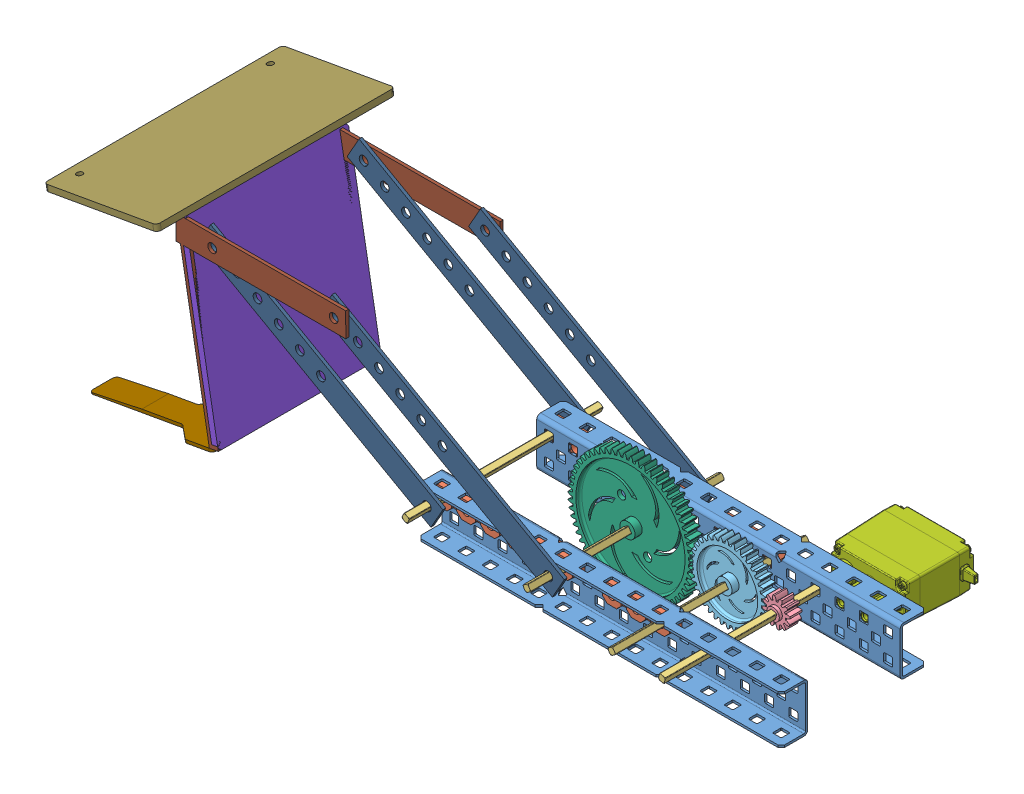
SolidWorks assembly LiftAssy, configuration Default. Lengths in mm.
Overall size (370.81 123.65 133.86).
26 component instances, 12 part files, 41 mates.
Components (placement in the parent):
- VL-CHAN-121-15 RevA-1: VL-CHAN-121-15 RevA [Default] at (-291.0348 35.1994 12.7) x (1 0 0) z (0 -1 0) size (190.5 13.87 25.4)
- VL-CHAN-121-15 RevA-2: VL-CHAN-121-15 RevA [Default] at (-153.4652 35.1994 63.5) x (-1 0 0) z (0 -1 0) size (190.5 13.87 25.4)
- BEARING-FLAT-1: BEARING-FLAT [Default] at (-272.0848 31.6992 -76.2762) x (0 0 1) z (0 -1 0) size (7.04 35.56 10.16)
- BEARING-FLAT-2: BEARING-FLAT [Default] at (-233.9848 31.8008 -76.2762) x (0 0 1) z (0 -1 0) size (7.04 35.56 10.16)
- BEARING-FLAT-3: BEARING-FLAT [Default] at (-183.1848 57.2008 152.4762) x (0 0 -1) z (0 1 0) size (7.04 35.56 10.16)
- BEARING-FLAT-4: BEARING-FLAT [Default] at (-235.9152 57.2008 -76.2762) x (0 0 1) z (0 1 0) size (7.04 35.56 10.16)
- BEARING-FLAT-5: BEARING-FLAT [Default] at (-233.9848 57.2008 152.4762) x (0 0 -1) z (0 1 0) size (7.04 35.56 10.16)
- BEARING-FLAT-6: BEARING-FLAT [Default] at (-272.0848 57.2008 152.4762) x (0 0 -1) z (0 1 0) size (7.04 35.56 10.16)
- SHAFT-4000-1: SHAFT-4000 [Default] at (-311.2008 44.5008 38.1) x (0.41269 0.910872 0) z (0 0 1) size (4.18 4.18 101.81)
- SHAFT-4000-2: SHAFT-4000 [Default] at (-247.7008 44.5008 38.1) x (0.537594 -0.843204 0) z (0 0 1) size (4.18 4.18 101.81)
- SHAFT-4000-3: SHAFT-4000 [Default] at (-196.9008 44.5008 44.45) x (0.810991 0.585059 0) z (0 0 1) size (4.18 4.18 101.81)
- SHAFT-4000-4: SHAFT-4000 [Default] at (-171.4187 44.4677 43.6) x (0.963526 -0.267616 0) z (0 0 1) size (4.18 4.18 101.81)
- VEX-12-TOOTH-GEAR-1: VEX-12-TOOTH-GEAR [Default] at (-171.388 44.4851 31.3309) x (0.963526 -0.267616 0) z (0 0 1) size (14.8 14.8 9.53)
- VEX-36-TOOTH-GEAR-1: VEX-36-TOOTH-GEAR [Default] at (-196.9357 44.5064 31.3309) x (0.810991 0.585059 0) z (0 0 1) size (40.08 40.08 9.53)
- VEX-60-TOOTH-GEAR-1: VEX-60-TOOTH-GEAR [Default] at (-247.7353 44.5084 31.3309) x (0.537594 -0.843204 0) z (0 0 1) size (65.54 65.54 9.53)
- VEX-2WIRE-MOTOR-1: VEX-2WIRE-MOTOR [Default] at (-160.3202 44.45 -30.5) x (-1 0 0) z (0 0 -1) size (46.4 20 51.81)
- Pyramid Intake-1: Pyramid Intake [Default] at (-392.6154 54.6194 -14.6496) x (0 0 1) z (-0.999593 -0.028533 0) size (125 114.43 256.59)
  - back-1: back [Default] at (51.2746 60.8094 41.9933) x (1 0 0) z (0 -0.146963 0.989142) size (85.5 99.5 3.17)
  - BottomForklift-1: BottomForklift [Default] at (51.2746 -39.6471 30.2777) x (1 0 0) z (0 -0.146963 0.989142) size (85.5 1.59 73.7)
  - Circles 5.5in Inch Shaft Bar-1: Circles 5.5in Inch Shaft Bar [Default] at (90.8496 -1.2906 -50.3225) x (0 0.85685 -0.515566) z (0 -0.515566 -0.85685) size (12.7 1.59 139.7)
  - Circles 5.5in Inch Shaft Bar-2: Circles 5.5in Inch Shaft Bar [Default] at (90.8496 -3.0112 -113.9492) x (0 0.85685 -0.515566) z (0 -0.515566 -0.85685) size (12.7 1.59 139.7)
  - Circles 5.5in Inch Shaft Bar-3: Circles 5.5in Inch Shaft Bar [Default] at (13.0621 -1.2906 -50.3225) x (0 0.85685 -0.515566) z (0 -0.515566 -0.85685) size (12.7 1.59 139.7)
  - Circles 5.5in Inch Shaft Bar-4: Circles 5.5in Inch Shaft Bar [Default] at (13.0621 -3.0112 -113.9492) x (0 0.85685 -0.515566) z (0 -0.515566 -0.85685) size (12.7 1.59 139.7)
  - Circles 3.5 inch Linkage-3: Circles 3.5 inch Linkage [Default] at (94.0246 47.7557 59.6803) x (0 0.999635 -0.027032) z (0 0.027032 0.999635) size (97.99 1.59 88.9)
  - Circles 3.5 inch Linkage-4: Circles 3.5 inch Linkage [Default] at (13.0621 47.7557 59.6803) x (0 0.999635 -0.027032) z (0 0.027032 0.999635) size (97.99 1.59 88.9)
  - top-2: top [Default] at (45.9604 60.8094 41.9933) x (1 0 0) z (0 -0.146963 0.989142) size (125 3.17 60)
Mates (geometry in assembly coordinates):
- Coincident7: coincident aligned: line of VL-CHAN-121-15 RevA-1 through (-312.9534 42.1386 12.7) axis (1 0 0); line of BEARING-FLAT-1 through (-312.9537 42.1386 12.7) axis (1 0 0)
- Coincident8: coincident aligned: line of VL-CHAN-121-15 RevA-1 through (-313.4614 46.2534 12.7) axis (0 -1 0); line of BEARING-FLAT-1 through (-313.4614 43.4086 12.7) axis (0 -1 0)
- Coincident9: coincident aligned: line of VL-CHAN-121-15 RevA-1 through (-275.3614 46.2534 12.7) axis (0 -1 0); line of BEARING-FLAT-2 through (-275.3614 43.5102 12.7) axis (0 -1 0)
- Coincident11: coincident aligned: line of VL-CHAN-121-15 RevA-1 through (-271.2466 46.7614 12.7) axis (-1 0 0); line of BEARING-FLAT-2 through (-274.0914 46.7614 12.7) axis (-1 0 0)
- Coincident17: coincident aligned: line of VL-CHAN-121-15 RevA-1 through (-233.1466 46.7614 12.7) axis (-1 0 0); line of BEARING-FLAT-4 through (-223.1898 46.7614 12.7) axis (-1 0 0)
- Coincident18: coincident aligned: line of VL-CHAN-121-15 RevA-2 through (-313.4614 42.6466 63.5) axis (0 1 0); line of BEARING-FLAT-6 through (-313.4614 42.7479 63.5) axis (0 1 0)
- Coincident19: coincident aligned: line of VL-CHAN-121-15 RevA-2 through (-312.9534 46.7614 63.5) axis (1 0 0); line of BEARING-FLAT-6 through (-312.9537 46.7614 63.5) axis (1 0 0)
- Coincident20: coincident aligned: line of VL-CHAN-121-15 RevA-2 through (-275.3614 42.6466 63.5) axis (0 1 0); line of BEARING-FLAT-5 through (-275.3614 42.7479 63.5) axis (0 1 0)
- Coincident21: coincident aligned: line of VL-CHAN-121-15 RevA-2 through (-274.8534 46.7614 63.5) axis (1 0 0); line of BEARING-FLAT-5 through (-274.8537 46.7614 63.5) axis (1 0 0)
- Coincident23: coincident aligned: line of VL-CHAN-121-15 RevA-2 through (-236.7534 46.7614 63.5) axis (1 0 0); line of BEARING-FLAT-3 through (-224.0537 46.7614 63.5) axis (1 0 0)
- Width1: width: plane of SHAFT-4000-1 through (-310.4099 42.3996 88.9) normal (-0.41269 -0.910872 0); plane of SHAFT-4000-1 through (-309.0997 45.2917 88.9) normal (0.41269 0.910872 0); cylinder of BEARING-FLAT-6 through (-311.2008 44.5008 69.85) axis (0 0 -1) radius 2.1209
- Width2: width: plane of SHAFT-4000-1 through (-313.302 43.7099 88.9) normal (-0.910872 0.41269 0); plane of SHAFT-4000-1 through (-310.4099 42.3996 88.9) normal (0.910872 -0.41269 0); cylinder of BEARING-FLAT-6 through (-311.2008 44.5008 69.85) axis (0 0 -1) radius 2.1209
- Distance1: distance = 25.4 mm aligned: plane of SHAFT-4000-1 through (-313.302 43.7099 88.9) normal (0 0 1); plane of VL-CHAN-121-15 RevA-2 through (-127 25.4 63.5) normal (0 0 1)
- Width3: width: plane of SHAFT-4000-2; plane of SHAFT-4000-2; cylinder of BEARING-FLAT-5 through (-247.7008 44.5008 69.85) axis (0 0 -1) radius 2.1209
- Width4: width: plane of SHAFT-4000-2; plane of SHAFT-4000-2; cylinder of BEARING-FLAT-5 through (-247.7008 44.5008 69.85) axis (0 0 -1) radius 2.1209
- Distance2: distance = 25.4 mm aligned: plane of SHAFT-4000-2 through (-247.2156 46.6928 88.9) normal (0 0 1); plane of VL-CHAN-121-15 RevA-2 through (-127 25.4 63.5) normal (0 0 1)
- Coincident24: coincident anti-aligned: plane of SHAFT-4000-2; plane of VEX-60-TOOTH-GEAR-1
- Coincident25: coincident anti-aligned: plane of SHAFT-4000-2; plane of VEX-60-TOOTH-GEAR-1
- Distance3: distance = 12.7 mm anti-aligned: plane of VEX-60-TOOTH-GEAR-1 through (-247.7353 44.5084 26.5684) normal (0 0 -1); plane of VL-CHAN-121-15 RevA-1 through (-317.5 25.4 13.8684) normal (0 0 1)
- Coincident28: coincident aligned: line of VL-CHAN-121-15 RevA-2 through (-199.1614 42.6466 63.5) axis (0 1 0); line of BEARING-FLAT-3 through (-199.1614 42.7479 63.5) axis (0 1 0)
- Coincident29: coincident aligned: line of VL-CHAN-121-15 RevA-1 through (-194.5386 42.6466 12.7) axis (0 1 0); line of BEARING-FLAT-4 through (-194.5386 42.7479 12.7) axis (0 1 0)
- Width5: width: plane of SHAFT-4000-3 through (-197.2595 42.2846 95.25) normal (-0.810991 -0.585059 0); plane of SHAFT-4000-3 through (-194.6846 44.1421 95.25) normal (0.810991 0.585059 0); cylinder of BEARING-FLAT-3 through (-196.9008 44.5008 69.85) axis (0 0 -1) radius 2.1209
- Width6: width: plane of SHAFT-4000-3 through (-199.117 44.8595 95.25) normal (-0.585059 0.810991 0); plane of SHAFT-4000-3 through (-197.2595 42.2846 95.25) normal (0.585059 -0.810991 0); cylinder of BEARING-FLAT-3 through (-196.9008 44.5008 69.85) axis (0 0 -1) radius 2.1209
- Distance4: distance = 25.4 mm aligned: plane of BEARING-FLAT-3 through (-215.6971 38.5377 69.85) normal (0 0 1); plane of SHAFT-4000-3 through (-199.117 44.8595 95.25) normal (0 0 1)
- Coincident30: coincident anti-aligned: plane of SHAFT-4000-3 through (-197.2595 42.2846 95.25) normal (0.585059 -0.810991 0); plane of VEX-36-TOOTH-GEAR-1 through (-197.3 42.2553 37.0459) normal (-0.585059 0.810991 0)
- Coincident31: coincident anti-aligned: plane of SHAFT-4000-3 through (-194.6846 44.1421 95.25) normal (0.810991 0.585059 0); plane of VEX-36-TOOTH-GEAR-1 through (-194.6846 44.1421 37.0459) normal (-0.810991 -0.585059 0)
- Distance5: distance = 12.7 mm anti-aligned: plane of VEX-36-TOOTH-GEAR-1 through (-196.9357 44.5064 26.5684) normal (0 0 -1); plane of VL-CHAN-121-15 RevA-1 through (-317.5 25.4 13.8684) normal (0 0 1)
- Coincident33: coincident anti-aligned: plane of VL-CHAN-121-15 RevA-1 through (-317.5 25.4 12.7) normal (0 0 -1); plane of VEX-2WIRE-MOTOR-1 through (-160.3202 44.45 12.7) normal (0 0 1)
- Parallel4: parallel anti-aligned: line of VL-CHAN-121-15 RevA-1 through (-188.473 50.8 0) axis (1 0 0); line of VEX-2WIRE-MOTOR-1 through (-141.8435 53.9263 -10.5) axis (-1 0 0)
- Width7: width: plane of VL-CHAN-121-15 RevA-1 through (-161.0614 46.7614 11.3284) normal (1 0 0); plane of VL-CHAN-121-15 RevA-1 through (-156.4386 46.7614 11.3284) normal (-1 0 0); cone of VEX-2WIRE-MOTOR-1 through (-158.75 44.45 -2.0131) axis (0 0 1)
- Coincident34: coincident anti-aligned: plane of SHAFT-4000-4 through (-172.5235 46.4221 94.4) normal (0.267616 0.963526 0); plane of VEX-2WIRE-MOTOR-1 through (-172.5724 46.4357 -7.2) normal (-0.267616 -0.963526 0)
- Coincident35: coincident anti-aligned: plane of SHAFT-4000-4 through (-170.314 42.5132 94.4) normal (0.963526 -0.267616 0); plane of VEX-2WIRE-MOTOR-1 through (-169.4643 45.5724 -7.2) normal (-0.963526 0.267616 0)
- Coincident36: coincident anti-aligned: plane of SHAFT-4000-4 through (-172.5235 46.4221 -7.2) normal (0 0 -1); plane of VEX-2WIRE-MOTOR-1 through (-170.3276 42.4643 -7.2) normal (0 0 1)
- Width8: width: plane of VL-CHAN-121-15 RevA-1 through (-148.3614 46.7614 11.3284) normal (0 -1 0); plane of VL-CHAN-121-15 RevA-1 through (-148.3614 42.1386 11.3284) normal (0 1 0); cone of VEX-2WIRE-MOTOR-1 through (-146.05 44.45 -2.0131) axis (0 0 1)
- Coincident37: coincident anti-aligned: plane of SHAFT-4000-4 through (-173.3732 43.3629 94.4) normal (-0.267616 -0.963526 0); plane of VEX-12-TOOTH-GEAR-1 through (-173.3732 43.3629 37.0459) normal (0.267616 0.963526 0)
- Coincident38: coincident anti-aligned: plane of SHAFT-4000-4 through (-173.3732 43.3629 94.4) normal (-0.963526 0.267616 0); plane of VEX-12-TOOTH-GEAR-1 through (-172.5101 46.4703 37.0459) normal (0.963526 -0.267616 0)
- Distance6: distance = 12.7 mm anti-aligned: plane of VEX-12-TOOTH-GEAR-1 through (-171.388 44.4851 26.5684) normal (0 0 -1); plane of VL-CHAN-121-15 RevA-1 through (-317.5 25.4 13.8684) normal (0 0 1)
- Width9: width: plane of SHAFT-4000-1 through (-313.302 43.7099 88.9) normal (-0.910872 0.41269 0); plane of SHAFT-4000-1 through (-310.4099 42.3996 88.9) normal (0.910872 -0.41269 0); cylinder of Pyramid Intake-1/Circles 5.5in Inch Shaft Bar-1 through (-311.2008 44.5008 77.7875) axis (0 0 -1) radius 2.31
- Width11: width: plane of SHAFT-4000-1 through (-309.0997 45.2917 88.9) normal (0.41269 0.910872 0); plane of SHAFT-4000-1 through (-310.4099 42.3996 88.9) normal (-0.41269 -0.910872 0); cylinder of Pyramid Intake-1/Circles 5.5in Inch Shaft Bar-1 through (-311.2008 44.5008 77.7875) axis (0 0 -1) radius 2.31
- Distance7: distance = 12.7 mm anti-aligned: plane of Pyramid Intake-1/Circles 5.5in Inch Shaft Bar-1 through (-342.2766 54.7652 76.2) normal (0 0 -1); plane of VL-CHAN-121-15 RevA-2 through (-127 25.4 63.5) normal (0 0 1)
- Width14: width: plane of SHAFT-4000-2 through (-249.8928 44.986 88.9) normal (-0.537594 0.843204 0); plane of SHAFT-4000-2 through (-248.186 42.3088 88.9) normal (0.537594 -0.843204 0); cylinder of Pyramid Intake-1/Circles 5.5in Inch Shaft Bar-2 through (-247.5509 44.5964 77.7875) axis (0 0 -1) radius 2.31
